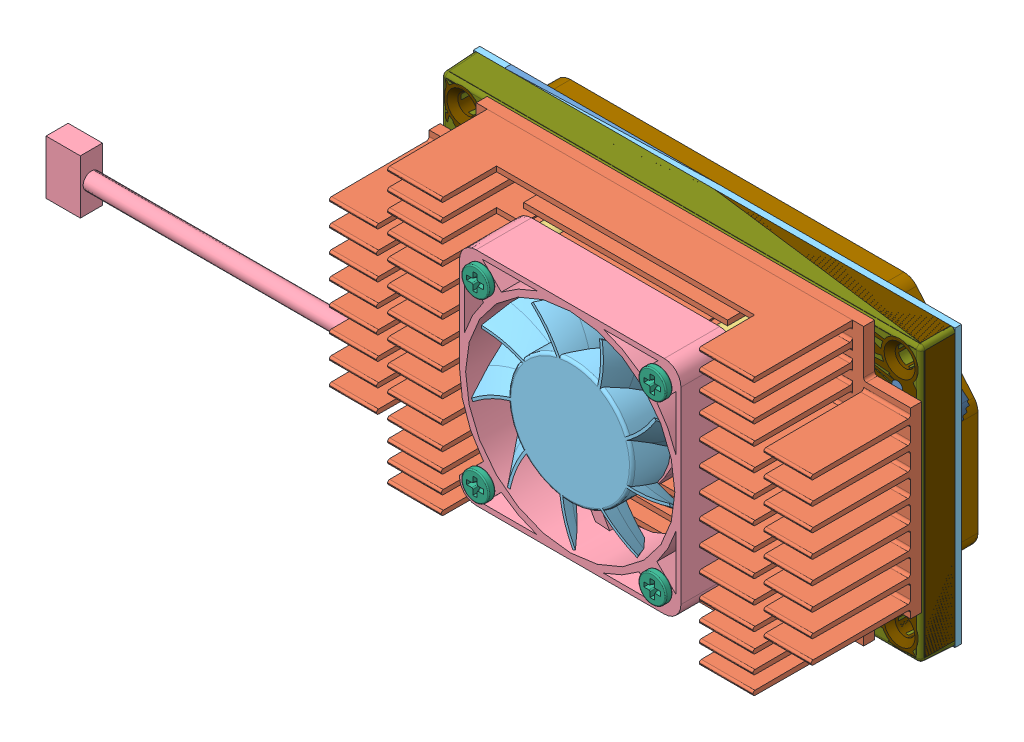
SolidWorks assembly JETSON-NEW_ASM, configuration Default. Lengths in mm. (continued)
Components (placement in the parent): (continued)
- 244-82180-1000-A01-07-31-15_ASM-1: 244-82180-1000-A01-07-31-15_ASM [Default] at origin size (87 50 8.3) (continued)
  - 039-0145-000_2-6: 039-0145-000_2 [Default] at (33.873 25.024 0) x (1 0 0) z (0 0 -1) size (1.4 0.7 0.62)
  - 039-0145-000_2-7: 039-0145-000_2 [Default] at (33.503 23.754 0) x (0 1 0) z (0 0 -1) size (1.4 0.7 0.62)
  - 039-0145-000_2-8: 039-0145-000_2 [Default] at (36.784 26.168 0) x (0 1 0) z (0 0 -1) size (1.4 0.7 0.62)
  - 039-0145-000_2-9: 039-0145-000_2 [Default] at (38.374 24.389 0) x (-1 0 0) z (0 0 -1) size (1.4 0.7 0.62)
  - 039-0188-000_3-5: 039-0188-000_3 [Default] at (36.3 38.2 0) x (-1 0 0) z (0 0 -1) size (1.4 0.7 0.67)
  - 039-0188-000_3-6: 039-0188-000_3 [Default] at (36.25 36.2 0) x (-1 0 0) z (0 0 -1) size (1.4 0.7 0.67)
  - 039-0188-000_3-7: 039-0188-000_3 [Default] at (36.9 32.05 0) x (-1 0 0) z (0 0 -1) size (1.4 0.7 0.67)
  - 039-0188-000_3-8: 039-0188-000_3 [Default] at (39.373 40.784 0) x (0 -1 0) z (0 0 -1) size (1.4 0.7 0.67)
  - 039-0145-000_2-10: 039-0145-000_2 [Default] at (39.753 24.004 0) x (0 1 0) z (0 0 -1) size (1.4 0.7 0.62)
  - 039-0145-000_2-11: 039-0145-000_2 [Default] at (39.495 25.352 0) x (1 0 0) z (0 0 -1) size (1.4 0.7 0.62)
  - 039-0188-000_3-9: 039-0188-000_3 [Default] at (38.003 41.604 0) x (0 1 0) z (0 0 -1) size (1.4 0.7 0.67)
  - 039-0145-000_2-12: 039-0145-000_2 [Default] at (41.353 24.824 0) x (0 1 0) z (0 0 -1) size (1.4 0.7 0.62)
  - 039-0145-000_2-13: 039-0145-000_2 [Default] at (43.188 24.838 0) x (0 1 0) z (0 0 -1) size (1.4 0.7 0.62)
  - 039-0145-000_2-14: 039-0145-000_2 [Default] at (42.268 24.828 0) x (0 1 0) z (0 0 -1) size (1.4 0.7 0.62)
  - 039-0145-000_2-15: 039-0145-000_2 [Default] at (42.863 23.214 0) x (1 0 0) z (0 0 -1) size (1.4 0.7 0.62)
  - 039-0197-000_3-1: 039-0197-000_3 [Default] at (48.75 34.85 0) x (1 0 0) z (0 0 -1) size (1.4 0.7 0.72)
  - 039-0197-000_3-2: 039-0197-000_3 [Default] at (47.5 35.75 0) x (1 0 0) z (0 0 -1) size (1.4 0.7 0.72)
  - 039-0188-000_3-10: 039-0188-000_3 [Default] at (45.093 41.024 0) x (1 0 0) z (0 0 -1) size (1.4 0.7 0.67)
  - 039-0197-000_3-3: 039-0197-000_3 [Default] at (45.9 35.75 0) x (-1 0 0) z (0 0 -1) size (1.4 0.7 0.72)
  - 039-0188-000_3-11: 039-0188-000_3 [Default] at (44.443 37.824 0) x (0 1 0) z (0 0 -1) size (1.4 0.7 0.67)
  - 039-0188-000_3-12: 039-0188-000_3 [Default] at (44.45 35.1 0) x (0 -1 0) z (0 0 -1) size (1.4 0.7 0.67)
  - 039-0188-000_3-13: 039-0188-000_3 [Default] at (11.15 20.65 0) x (0 1 0) z (0 0 -1) size (1.4 0.7 0.67)
  - 039-0145-000_2-16: 039-0145-000_2 [Default] at (11.607 27.979 1.164) x (-1 0 0) z (0 0 1) size (1.4 0.7 0.62)
  - 039-0145-000_2-17: 039-0145-000_2 [Default] at (16.618 28.397 1.164) size (1.4 0.7 0.62)
  - 039-0145-000_2-18: 039-0145-000_2 [Default] at (28.65 14.4 0) x (0 -1 0) z (0 0 -1) size (1.4 0.7 0.62)
  - 039-0145-000_2-19: 039-0145-000_2 [Default] at (6.05 21.2 0) x (-1 0 0) z (0 0 -1) size (1.4 0.7 0.62)
  - 039-0145-000_2-20: 039-0145-000_2 [Default] at (29.763 16.794 0) x (0 1 0) z (0 0 -1) size (1.4 0.7 0.62)
  - 039-0145-000_2-21: 039-0145-000_2 [Default] at (29.933 14.994 0) x (-1 0 0) z (0 0 -1) size (1.4 0.7 0.62)
  - 039-0145-000_2-22: 039-0145-000_2 [Default] at (28.85 20.15 0) x (1 0 0) z (0 0 -1) size (1.4 0.7 0.62)
  - 039-0145-000_2-23: 039-0145-000_2 [Default] at (31.063 15.984 0) x (-1 0 0) z (0 0 -1) size (1.4 0.7 0.62)
  - 039-0145-000_2-24: 039-0145-000_2 [Default] at (31.063 16.894 0) x (-1 0 0) z (0 0 -1) size (1.4 0.7 0.62)
  - 039-0145-000_2-25: 039-0145-000_2 [Default] at (31.703 12.644 0) x (0 -1 0) z (0 0 -1) size (1.4 0.7 0.62)
  - 039-0145-000_2-26: 039-0145-000_2 [Default] at (30.443 12.584 0) x (-1 0 0) z (0 0 -1) size (1.4 0.7 0.62)
  - 039-0145-000_2-27: 039-0145-000_2 [Default] at (30.443 13.484 0) x (-1 0 0) z (0 0 -1) size (1.4 0.7 0.62)
  - 039-0145-000_2-28: 039-0145-000_2 [Default] at (33 11.85 0) x (1 0 0) z (0 0 -1) size (1.4 0.7 0.62)
  - 039-0145-000_2-29: 039-0145-000_2 [Default] at (29.75 11.65 0) x (-1 0 0) z (0 0 -1) size (1.4 0.7 0.62)
  - 039-0145-000_2-30: 039-0145-000_2 [Default] at (29.413 21.065 0) x (1 0 0) z (0 0 -1) size (1.4 0.7 0.62)
  - 039-0145-000_2-31: 039-0145-000_2 [Default] at (34.423 13.174 0) x (0 -1 0) z (0 0 -1) size (1.4 0.7 0.62)
  - 039-0188-000_3-14: 039-0188-000_3 [Default] at (35.323 13.174 0) x (0 -1 0) z (0 0 -1) size (1.4 0.7 0.67)
  - 039-0145-000_2-32: 039-0145-000_2 [Default] at (34.963 11.574 0) x (0 -1 0) z (0 0 -1) size (1.4 0.7 0.62)
  - 039-0145-000_2-33: 039-0145-000_2 [Default] at (32.323 18.454 0) x (0 -1 0) z (0 0 -1) size (1.4 0.7 0.62)
  - 039-0145-000_2-34: 039-0145-000_2 [Default] at (33.523 13.124 0) x (0 -1 0) z (0 0 -1) size (1.4 0.7 0.62)
  - 039-0145-000_2-35: 039-0145-000_2 [Default] at (32.623 13.124 0) x (0 -1 0) z (0 0 -1) size (1.4 0.7 0.62)
  - 039-0145-000_2-36: 039-0145-000_2 [Default] at (30.888 22.484 0) x (-1 0 0) z (0 0 -1) size (1.4 0.7 0.62)
  - 039-0145-000_2-37: 039-0145-000_2 [Default] at (31.043 21.054 0) x (-1 0 0) z (0 0 -1) size (1.4 0.7 0.62)
  - 039-0145-000_2-38: 039-0145-000_2 [Default] at (31.063 19.634 0) x (-1 0 0) z (0 0 -1) size (1.4 0.7 0.62)
  - 039-0145-000_2-39: 039-0145-000_2 [Default] at (31.063 18.724 0) x (-1 0 0) z (0 0 -1) size (1.4 0.7 0.62)
  - 039-0145-000_2-40: 039-0145-000_2 [Default] at (31.063 17.794 0) x (-1 0 0) z (0 0 -1) size (1.4 0.7 0.62)
  - 039-0145-000_2-41: 039-0145-000_2 [Default] at (38.263 21.414 0) x (0 -1 0) z (0 0 -1) size (1.4 0.7 0.62)
  - 039-0145-000_2-42: 039-0145-000_2 [Default] at (37.353 21.374 0) x (0 -1 0) z (0 0 -1) size (1.4 0.7 0.62)
  - 039-0145-000_2-43: 039-0145-000_2 [Default] at (38.803 19.694 0) x (0 -1 0) z (0 0 -1) size (1.4 0.7 0.62)
  - 039-0145-000_2-44: 039-0145-000_2 [Default] at (37.853 19.694 0) x (0 -1 0) z (0 0 -1) size (1.4 0.7 0.62)
  - 039-0145-000_2-45: 039-0145-000_2 [Default] at (38.758 15.717 0) x (0 -1 0) z (0 0 -1) size (1.4 0.7 0.62)
  - 039-0145-000_2-46: 039-0145-000_2 [Default] at (37.846 15.717 0) x (0 -1 0) z (0 0 -1) size (1.4 0.7 0.62)
  - 039-0145-000_2-47: 039-0145-000_2 [Default] at (33.659 19.074 0) x (1 0 0) z (0 0 -1) size (1.4 0.7 0.62)
  - 039-0145-000_2-48: 039-0145-000_2 [Default] at (38.723 13.214 0) x (0 -1 0) z (0 0 -1) size (1.4 0.7 0.62)
  - 039-0145-000_2-49: 039-0145-000_2 [Default] at (38.003 11.924 0) x (1 0 0) z (0 0 -1) size (1.4 0.7 0.62)
  - 039-0145-000_2-50: 039-0145-000_2 [Default] at (36.073 19.694 0) x (0 -1 0) z (0 0 -1) size (1.4 0.7 0.62)
  - 039-0145-000_2-51: 039-0145-000_2 [Default] at (36.42 18.444 0) x (-1 0 0) z (0 0 -1) size (1.4 0.7 0.62)
  - 039-0145-000_2-52: 039-0145-000_2 [Default] at (36.42 16.644 0) x (-1 0 0) z (0 0 -1) size (1.4 0.7 0.62)
  - 039-0145-000_2-53: 039-0145-000_2 [Default] at (36.42 17.544 0) x (-1 0 0) z (0 0 -1) size (1.4 0.7 0.62)
  - 039-0145-000_2-54: 039-0145-000_2 [Default] at (37.123 13.174 0) x (0 -1 0) z (0 0 -1) size (1.4 0.7 0.62)
  - 039-0145-000_2-55: 039-0145-000_2 [Default] at (36.343 11.924 0) x (1 0 0) z (0 0 -1) size (1.4 0.7 0.62)
  - 039-0145-000_2-56: 039-0145-000_2 [Default] at (33.713 21.724 0) x (1 0 0) z (0 0 -1) size (1.4 0.7 0.62)
  - 039-0145-000_2-57: 039-0145-000_2 [Default] at (35.005 19.699 0) x (0 1 0) z (0 0 -1) size (1.4 0.7 0.62)
  - 039-0145-000_2-58: 039-0145-000_2 [Default] at (33.743 19.974 0) x (1 0 0) z (0 0 -1) size (1.4 0.7 0.62)
  - 039-0145-000_2-59: 039-0145-000_2 [Default] at (33.663 18.174 0) x (1 0 0) z (0 0 -1) size (1.4 0.7 0.62)
  - 039-0145-000_2-60: 039-0145-000_2 [Default] at (33.663 17.274 0) x (1 0 0) z (0 0 -1) size (1.4 0.7 0.62)
  - 039-0145-000_2-61: 039-0145-000_2 [Default] at (41.223 12.474 0) x (0 -1 0) z (0 0 -1) size (1.4 0.7 0.62)
  - 039-0145-000_2-62: 039-0145-000_2 [Default] at (42.133 12.464 0) x (0 -1 0) z (0 0 -1) size (1.4 0.7 0.62)
  - 039-0145-000_2-63: 039-0145-000_2 [Default] at (41.243 11.194 0) x (1 0 0) z (0 0 -1) size (1.4 0.7 0.62)
  - 039-0145-000_2-64: 039-0145-000_2 [Default] at (39.173 21.394 0) x (0 -1 0) z (0 0 -1) size (1.4 0.7 0.62)
  - 039-0145-000_2-65: 039-0145-000_2 [Default] at (40.513 19.724 0) x (0 -1 0) z (0 0 -1) size (1.4 0.7 0.62)
  - 039-0145-000_2-66: 039-0145-000_2 [Default] at (39.859 15.764 0) x (0 1 0) z (0 0 -1) size (1.4 0.7 0.62)
  - 039-0145-000_2-67: 039-0145-000_2 [Default] at (39.623 13.134 0) x (0 -1 0) z (0 0 -1) size (1.4 0.7 0.62)
  - 039-0145-000_2-68: 039-0145-000_2 [Default] at (39.973 11.514 0) x (0 -1 0) z (0 0 -1) size (1.4 0.7 0.62)
  - 039-0145-000_2-69: 039-0145-000_2 [Default] at (42.613 22.304 0) x (1 0 0) z (0 0 -1) size (1.4 0.7 0.62)
  - 039-0145-000_2-70: 039-0145-000_2 [Default] at (42.743 19.696 0) x (0 -1 0) z (0 0 -1) size (1.4 0.7 0.62)
  - 039-0145-000_2-71: 039-0145-000_2 [Default] at (42.143 17.394 0) x (1 0 0) z (0 0 -1) size (1.4 0.7 0.62)
  - 039-0145-000_2-72: 039-0145-000_2 [Default] at (42.163 16.484 0) x (1 0 0) z (0 0 -1) size (1.4 0.7 0.62)
  - 039-0145-000_2-73: 039-0145-000_2 [Default] at (42.183 15.564 0) x (1 0 0) z (0 0 -1) size (1.4 0.7 0.62)
  - 039-0145-000_2-74: 039-0145-000_2 [Default] at (42.163 14.634 0) x (1 0 0) z (0 0 -1) size (1.4 0.7 0.62)
  - 039-0145-000_2-75: 039-0145-000_2 [Default] at (43.033 13.374 0) x (0 1 0) z (0 0 -1) size (1.4 0.7 0.62)
  - 039-0145-000_2-76: 039-0145-000_2 [Default] at (40.433 21.064 0) x (-1 0 0) z (0 0 -1) size (1.4 0.7 0.62)
  - 039-0188-000_3-15: 039-0188-000_3 [Default] at (43.796 15.444 0) x (1 0 0) z (0 0 -1) size (1.4 0.7 0.67)
  - 039-0145-000_2-77: 039-0145-000_2 [Default] at (57 41.1 1.164) x (-1 0 0) z (0 0 1) size (1.4 0.7 0.62)
  - 039-0145-000_2-78: 039-0145-000_2 [Default] at (69.75 34.15 0) x (0 -1 0) z (0 0 -1) size (1.4 0.7 0.62)
  - 039-0188-000_3-16: 039-0188-000_3 [Default] at (72.05 30.95 0) x (-1 0 0) z (0 0 -1) size (1.4 0.7 0.67)
  - 039-0188-000_3-17: 039-0188-000_3 [Default] at (74.4 31.9 0) x (1 0 0) z (0 0 -1) size (1.4 0.7 0.67)
  - 039-0145-000_2-79: 039-0145-000_2 [Default] at (72.753 31.884 0) x (1 0 0) z (0 0 -1) size (1.4 0.7 0.62)
  - 039-0145-000_2-80: 039-0145-000_2 [Default] at (19.986 32.449 0) x (1 0 0) z (0 0 -1) size (1.4 0.7 0.62)
  - 039-0145-000_2-81: 039-0145-000_2 [Default] at (35.043 22.074 0) x (0 -1 0) z (0 0 -1) size (1.4 0.7 0.62)
  - 039-0145-000_2-82: 039-0145-000_2 [Default] at (29.622 22.319 0) x (0 1 0) z (0 0 -1) size (1.4 0.7 0.62)
  - 091-0022-000_1-1: 091-0022-000_1 [Default] at (69.45 12.65 0) x (1 0 0) z (0 0 -1) size (2 2.51 1.1)
  - 091-0022-000_1-2: 091-0022-000_1 [Default] at (59.9 10.85 1.164) x (0 1 0) z (0 0 1) size (2 2.51 1.1)
  - 300-0405-000_1-1: 300-0405-000_1 [Default] at (71.98 12.636 0) x (-1 0 0) z (0 0 -1) size (2 2.51 0.9)
  - 130-0580-000_4-1: 130-0580-000_4 [Default] at (59.063 24.389 1.164) x (-1 0 0) z (0 0 1) size (4.96 4.06 2)
  - 130-0580-000_4-2: 130-0580-000_4 [Default] at (59.063 15.039 1.164) x (-1 0 0) z (0 0 1) size (4.96 4.06 2)
  - 032-0470-000_2-1: 032-0470-000_2 [Default] at (69.75 32.2 0) x (0 -1 0) z (0 0 -1) size (2 0.84 0.97)
  - 032-0470-000_2-2: 032-0470-000_2 [Default] at (68.7 35.2 0) x (0 1 0) z (0 0 -1) size (2 0.84 0.97)
  - 032-0470-000_2-3: 032-0470-000_2 [Default] at (76.75 34.8 0) x (0 1 0) z (0 0 -1) size (2 0.84 0.97)
  - 032-0470-000_2-4: 032-0470-000_2 [Default] at (76.75 32.55 0) x (0 -1 0) z (0 0 -1) size (2 0.84 0.97)
  - 032-0421-000_2-1: 032-0421-000_2 [Default] at (67.6 18.85 1.164) x (-1 0 0) z (0 0 1) size (2 0.84 0.93)
  - 032-0421-000_2-2: 032-0421-000_2 [Default] at (72.4 14.7 1.164) size (2 0.84 0.93)
  - 032-0421-000_2-3: 032-0421-000_2 [Default] at (72.4 15.8 1.164) size (2 0.84 0.93)
  - 032-0421-000_2-4: 032-0421-000_2 [Default] at (72.4 16.9 1.164) size (2 0.84 0.93)
  - 032-0421-000_2-5: 032-0421-000_2 [Default] at (69.256 18.703 1.164) x (0 1 0) z (0 0 1) size (2 0.84 0.93)
  - 032-0421-000_2-6: 032-0421-000_2 [Default] at (71.8 26.54 1.164) x (0 1 0) z (0 0 1) size (2 0.84 0.93)
  - 032-0421-000_2-7: 032-0421-000_2 [Default] at (72.57 24.76 1.164) size (2 0.84 0.93)
  - 032-0421-000_2-8: 032-0421-000_2 [Default] at (72.593 21.459 1.164) size (2 0.84 0.93)
  - 032-0421-000_2-9: 032-0421-000_2 [Default] at (72.593 22.559 1.164) size (2 0.84 0.93)
  - 032-0421-000_2-10: 032-0421-000_2 [Default] at (72.593 23.659 1.164) size (2 0.84 0.93)
  - 032-0421-000_2-11: 032-0421-000_2 [Default] at (72.65 19.8 1.164) x (0 1 0) z (0 0 1) size (2 0.84 0.93)
  - 032-0421-000_2-12: 032-0421-000_2 [Default] at (70.61 25.68 1.164) x (0 1 0) z (0 0 1) size (2 0.84 0.93)
  - 032-0421-000_2-13: 032-0421-000_2 [Default] at (69.5 25.68 1.164) x (0 1 0) z (0 0 1) size (2 0.84 0.93)
  - 032-0421-000_2-14: 032-0421-000_2 [Default] at (71.553 19.804 1.164) x (0 1 0) z (0 0 1) size (2 0.84 0.93)
  - 032-0421-000_2-15: 032-0421-000_2 [Default] at (68.39 25.68 1.164) x (0 1 0) z (0 0 1) size (2 0.84 0.93)
  - 032-0421-000_2-16: 032-0421-000_2 [Default] at (70.35 19.8 1.164) x (0 1 0) z (0 0 1) size (2 0.84 0.93)
  - 036-0034-000_1-1: 036-0034-000_1 [Default] at (75.23 38.16 1.164) x (-1 0 0) z (0 0 1) size (2 0.84 1.02)
  - 036-0034-000_1-2: 036-0034-000_1 [Default] at (2.62 13.59 1.164) x (-1 0 0) z (0 0 1) size (2 0.84 1.02)
  - 039-0168-000_1-1: 039-0168-000_1 [Default] at (39.23 17.12 0) x (1 0 0) z (0 0 -1) size (2 0.84 0.92)
  - 039-0168-000_1-2: 039-0168-000_1 [Default] at (43.593 17.044 0) x (0 -1 0) z (0 0 -1) size (2 0.84 0.92)
  - 039-0168-000_1-3: 039-0168-000_1 [Default] at (45.6 19.3 0) x (0 1 0) z (0 0 -1) size (2 0.84 0.92)
  - 039-0168-000_1-4: 039-0168-000_1 [Default] at (46.75 19.3 0) x (0 1 0) z (0 0 -1) size (2 0.84 0.92)
  - 039-0168-000_1-5: 039-0168-000_1 [Default] at (44.693 17.044 0) x (0 -1 0) z (0 0 -1) size (2 0.84 0.92)
  - 039-0125-000_1-1: 039-0125-000_1 [Default] at (57.653 33.054 1.164) size (2 0.84 0.97)
  - 039-0125-000_1-2: 039-0125-000_1 [Default] at (58.453 14.204 0) x (0 -1 0) z (0 0 -1) size (2 0.84 0.97)
  - 032-0056-000_2-1: 032-0056-000_2 [Default] at (55.353 40.004 1.164) size (2 0.84 1.02)
  - 039-0125-000_1-3: 039-0125-000_1 [Default] at (55.67 36.86 1.164) x (0 -1 0) z (0 0 1) size (2 0.84 0.97)
  - 039-0125-000_1-4: 039-0125-000_1 [Default] at (55.67 34.6 1.164) x (0 1 0) z (0 0 1) size (2 0.84 0.97)
  - 032-0056-000_2-2: 032-0056-000_2 [Default] at (54.489 31.838 1.164) size (2 0.84 1.02)
  - 032-0056-000_2-3: 032-0056-000_2 [Default] at (55.145 29.717 1.164) x (0 1 0) z (0 0 1) size (2 0.84 1.02)
  - 039-0125-000_1-5: 039-0125-000_1 [Default] at (59.953 33.054 1.164) x (-1 0 0) z (0 0 1) size (2 0.84 0.97)
  - 032-0056-000_2-4: 032-0056-000_2 [Default] at (59.62 31.466 0) x (1 0 0) z (0 0 -1) size (2 0.84 1.02)
  - 039-0125-000_1-6: 039-0125-000_1 [Default] at (61.796 34.84 1.164) x (0 1 0) z (0 0 1) size (2 0.84 0.97)
  - 215-0151-000_1-1: 215-0151-000_1 [Default] at (61.52 33.156 0) x (1 0 0) z (0 0 -1) size (2 0.84 0.6)
  - 032-0056-000_2-5: 032-0056-000_2 [Default] at (61.873 31.574 1.164) x (-1 0 0) z (0 0 1) size (2 0.84 1.02)
  - 032-0056-000_2-6: 032-0056-000_2 [Default] at (62.63 29.916 1.164) x (0 -1 0) z (0 0 1) size (2 0.84 1.02)
  - 039-0125-000_1-7: 039-0125-000_1 [Default] at (65.253 22.254 0) x (-1 0 0) z (0 0 -1) size (2 0.84 0.97)
  - 039-0168-000_1-6: 039-0168-000_1 [Default] at (44.7 13.8 0) x (0 1 0) z (0 0 -1) size (2 0.84 0.92)
  - 039-0037-000_1-1: 039-0037-000_1 [Default] at (68.83 5.23 1.164) x (0 -1 0) z (0 0 1) size (2 0.84 1.02)
  - 039-0037-000_1-2: 039-0037-000_1 [Default] at (77.9 14.1 1.164) x (0 1 0) z (0 0 1) size (2 0.84 1.02)
  - 039-0037-000_1-3: 039-0037-000_1 [Default] at (75.8 4.05 1.164) size (2 0.84 1.02)
  - 195-1225-000_1-1: 195-1225-000_1 [Default] at (62.4 42.78 0) x (0 1 0) z (0 0 -1) size (2 0.84 0.62)
  - 195-1260-000_1-1: 195-1260-000_1 [Default] at (10.9 32.65 0) x (1 0 0) z (0 0 -1) size (2 0.84 0.62)
  - 036-0043-000_1-1: 036-0043-000_1 [Default] at (5.524 36.6 0) x (0 1 0) z (0 0 -1) size (2 0.84 1.02)
  - 100-0104-000_1-1: 100-0104-000_1 [Default] at (28.2 15.55 0) x (1 0 0) z (0 0 -1) size (1.75 0.53 0.5)
  - 100-0063-000_1-1: 100-0063-000_1 [Default] at (21.1 20.85 1.164) x (-1 0 0) z (0 0 1) size (1.75 0.53 0.55)
  - 100-0063-000_1-2: 100-0063-000_1 [Default] at (45.21 8.116 1.164) size (1.75 0.53 0.55)
  - 100-0063-000_1-3: 100-0063-000_1 [Default] at (21.8 29.4 1.164) x (0 1 0) z (0 0 1) size (1.75 0.53 0.55)
  - 100-0063-000_1-4: 100-0063-000_1 [Default] at (27.15 25.1 1.164) x (-1 0 0) z (0 0 1) size (1.75 0.53 0.55)
  - 100-0063-000_1-5: 100-0063-000_1 [Default] at (27.713 20.824 1.164) x (0 1 0) z (0 0 1) size (1.75 0.53 0.55)
  - 100-0063-000_1-6: 100-0063-000_1 [Default] at (32.232 9.282 1.164) size (1.75 0.53 0.55)
  - 100-0104-000_1-2: 100-0104-000_1 [Default] at (28.8 19.25 0) x (1 0 0) z (0 0 -1) size (1.75 0.53 0.5)
  - 100-0104-000_1-3: 100-0104-000_1 [Default] at (33.6 11.05 0) x (1 0 0) z (0 0 -1) size (1.75 0.53 0.5)
  - 100-0063-000_1-7: 100-0063-000_1 [Default] at (33.943 9.709 1.164) x (0 -1 0) z (0 0 1) size (1.75 0.53 0.55)
  - 100-0189-000_2-1: 100-0189-000_2 [Default] at (43.113 20.934 0) x (1 0 0) z (0 0 -1) size (1.75 0.53 0.55)
  - 100-0063-000_1-8: 100-0063-000_1 [Default] at (46.76 10.216 1.164) size (1.75 0.53 0.55)
  - 100-0189-000_2-2: 100-0189-000_2 [Default] at (22.95 25.35 1.164) x (-1 0 0) z (0 0 1) size (1.75 0.53 0.55)
  - 100-0063-000_1-9: 100-0063-000_1 [Default] at (46.93 23.266 1.164) size (1.75 0.53 0.55)
  - 100-0165-000_1-1: 100-0165-000_1 [Default] at (73.7 12.5 0) x (0 -1 0) z (0 0 -1) size (1.75 0.53 0.6)
  - 039-0122-000_1-1: 039-0122-000_1 [Default] at (53.84 22.3 0) x (0 -1 0) z (0 0 -1) size (3.05 1.27 0.95)
  - 039-0122-000_1-2: 039-0122-000_1 [Default] at (55.93 22.35 0) x (0 -1 0) z (0 0 -1) size (3.05 1.27 0.95)
  - 032-0037-000_2-1: 032-0037-000_2 [Default] at (47.8 13.8 0) x (1 0 0) z (0 0 -1) size (3.05 1.27 0.95)
  - 032-0037-000_2-2: 032-0037-000_2 [Default] at (40.15 26.75 0) x (1 0 0) z (0 0 -1) size (3.05 1.27 0.95)
  - 039-0122-000_1-3: 039-0122-000_1 [Default] at (47.153 31.164 0) x (0 1 0) z (0 0 -1) size (3.05 1.27 0.95)
  - 039-0122-000_1-4: 039-0122-000_1 [Default] at (48.803 31.154 0) x (0 1 0) z (0 0 -1) size (3.05 1.27 0.95)
  - 039-0122-000_1-5: 039-0122-000_1 [Default] at (47.278 13.804 1.164) x (0 -1 0) z (0 0 1) size (3.05 1.27 0.95)
  - 032-0037-000_2-3: 032-0037-000_2 [Default] at (47.778 15.548 0) x (1 0 0) z (0 0 -1) size (3.05 1.27 0.95)
  - 032-0037-000_2-4: 032-0037-000_2 [Default] at (48.978 13.804 1.164) x (0 -1 0) z (0 0 1) size (3.05 1.27 0.95)
  - 039-0122-000_1-6: 039-0122-000_1 [Default] at (49.67 20.36 0) x (1 0 0) z (0 0 -1) size (3.05 1.27 0.95)
  - 032-0037-000_2-5: 032-0037-000_2 [Default] at (47.778 17.15 0) x (1 0 0) z (0 0 -1) size (3.05 1.27 0.95)
  - 032-0037-000_2-6: 032-0037-000_2 [Default] at (50.678 13.804 1.164) x (0 -1 0) z (0 0 1) size (3.05 1.27 0.95)
  - 039-0122-000_1-7: 039-0122-000_1 [Default] at (59.544 23.53 0) x (1 0 0) z (0 0 -1) size (3.05 1.27 0.95)
  - 039-0122-000_1-8: 039-0122-000_1 [Default] at (57.95 28.15 1.164) size (3.05 1.27 0.95)
  - 039-0122-000_1-9: 039-0122-000_1 [Default] at (59.515 25.132 0) x (1 0 0) z (0 0 -1) size (3.05 1.27 0.95)
  - 039-0122-000_1-10: 039-0122-000_1 [Default] at (59.483 28.504 0) x (1 0 0) z (0 0 -1) size (3.05 1.27 0.95)
  - 039-0122-000_1-11: 039-0122-000_1 [Default] at (59.483 26.754 0) x (1 0 0) z (0 0 -1) size (3.05 1.27 0.95)
  - 039-0122-000_1-12: 039-0122-000_1 [Default] at (59.483 30.134 0) x (1 0 0) z (0 0 -1) size (3.05 1.27 0.95)
  - 215-0165-000_1-1: 215-0165-000_1 [Default] at (73.833 26.174 1.164) size (3.05 1.27 0.6)
  - 215-0165-000_1-2: 215-0165-000_1 [Default] at (74.004 19.147 1.164) x (0 1 0) z (0 0 1) size (3.05 1.27 0.6)
  - 032-0213-000_1-1: 032-0213-000_1 [Default] at (12.3 38.75 0) x (1 0 0) z (0 0 -1) size (3.05 1.27 1.45)
  - 100-0077-000_1-1: 100-0077-000_1 [Default] at (16.393 37.444 1.164) x (-1 0 0) z (0 0 1) size (2.22 0.81 0.95)
  - 085-0232-000_1-1: 085-0232-000_1 [Default] at (66.12 7.63 1.164) x (-1 0 0) z (0 0 1) size (3.81 2.5 0.75)
  - 161-0188-600_2-1: 161-0188-600_2 [Default] at (28.903 37.199 1.164) x (0 1 0) z (0 0 1) size (10.1 15.1 1)
  - 161-0188-600_2-2: 161-0188-600_2 [Default] at (44.603 37.199 1.164) x (0 1 0) z (0 0 1) size (10.1 15.1 1)
  - 300-0868-000_3-1: 300-0868-000_3 [Default] at (53.3 9.55 1.164) size (1 0.6 0.41)
  - 300-0868-000_3-2: 300-0868-000_3 [Default] at (15.5 12.85 0) x (-1 0 0) z (0 0 -1) size (1 0.6 0.41)
  - 300-0868-000_3-3: 300-0868-000_3 [Default] at (71 25.95 0) x (1 0 0) z (0 0 -1) size (1 0.6 0.41)
  - 300-0868-000_3-4: 300-0868-000_3 [Default] at (63.182 37.401 0) x (0 1 0) z (0 0 -1) size (1 0.6 0.41)
  - 300-0870-000_1-1: 300-0870-000_1 [Default] at (31.482 11.077 0) x (-1 0 0) z (0 0 -1) size (1 0.6 0.41)
  - 131-0632-000_2-1: 131-0632-000_2 [Default] at (72.11 12.9 1.164) size (3.05 1.27 1.4)
  - 300-0494-000_1-1: 300-0494-000_1 [Default] at (71.55 15.75 0) x (1 0 0) z (0 0 -1) size (2.94 3.2 1.21)
  - 305-0002-000_1-1: 305-0002-000_1 [Default] at (7.2 38.8 0) x (1 0 0) z (0 0 -1) size (2.94 3.2 1.12)
  - 091-0004-000_1-1: 091-0004-000_1 [Default] at (10.4 42.15 0) x (-1 0 0) z (0 0 -1) size (2.94 3.2 1.27)
  - 300-0329-000_1-1: 300-0329-000_1 [Default] at (72.34 28.306 0) x (1 0 0) z (0 0 -1) size (2.94 3.2 1.26)
  - 300-0329-000_1-2: 300-0329-000_1 [Default] at (64.59 42.16 0) x (-1 0 0) z (0 0 -1) size (2.94 3.2 1.26)
  - 300-0329-000_1-3: 300-0329-000_1 [Default] at (56.09 12.826 0) x (-1 0 0) z (0 0 -1) size (2.94 3.2 1.26)
  - 300-0329-000_1-4: 300-0329-000_1 [Default] at (65.57 37.196 0) x (1 0 0) z (0 0 -1) size (2.94 3.2 1.26)
  - 300-0329-000_1-5: 300-0329-000_1 [Default] at (65.72 33.816 0) x (0 -1 0) z (0 0 -1) size (2.94 3.2 1.26)
  - 300-0329-000_1-6: 300-0329-000_1 [Default] at (62.55 12.6 0) x (0 1 0) z (0 0 -1) size (2.94 3.2 1.26)
  - 300-0329-000_1-7: 300-0329-000_1 [Default] at (10.54 35.996 0) x (1 0 0) z (0 0 -1) size (2.94 3.2 1.26)
  - 080-0550-000_2-1: 080-0550-000_2 [Default] at (-1.294 28.232 1.164) x (0 1 0) z (0 0 1) size (3.63 4.07 1.47)
  - 080-0550-000_2-2: 080-0550-000_2 [Default] at (-1.294 33.789 1.164) x (0 1 0) z (0 0 1) size (3.63 4.07 1.47)
  - SAMTEC-SEAF-50-05-S-08-02-A-K_ASM-1: SAMTEC-SEAF-50-05-S-08-02-A-K_ASM [Default] at (39.4993 3.4 -0.7366) x (0 -1 0) z (1 0 0) size (10.74 6.33 70.16)
    - SAMTEC-JETSON_ASM-1: SAMTEC-JETSON_ASM [Default] at origin size (10.74 6.33 70.16)
      - BOSS-BASE-1: BOSS-BASE [Default] at origin size (10.74 6.33 70.16)
- 244-82180-1000-A03-10-12-15_ASM-1: 244-82180-1000-A03-10-12-15_ASM [Default] at origin size (87 50 8.3)
  - 142-82180-1000-A03-10-12-15-1: 142-82180-1000-A03-10-12-15 [Default] at origin size (87 50 1.16)
  - 032-0628-000_1-1: 032-0628-000_1 [Default] at (13.96 6.5 1.164) x (0 1 0) z (0 0 1) size (3.82 1.6 1.8)
  - 032-0628-000_1-2: 032-0628-000_1 [Default] at (11.83 6.48 1.164) x (0 1 0) z (0 0 1) size (3.82 1.6 1.8)
  - 032-0628-000_1-3: 032-0628-000_1 [Default] at (55.94 22.44 0) x (0 -1 0) z (0 0 -1) size (3.82 1.6 1.8)
  - 032-0628-000_1-4: 032-0628-000_1 [Default] at (53.83 22.43 0) x (0 -1 0) z (0 0 -1) size (3.82 1.6 1.8)
  - 032-0637-000_1-1: 032-0637-000_1 [Default] at (72.8 32.06 1.164) size (3.82 1.6 1.8)
  - 032-0637-000_1-2: 032-0637-000_1 [Default] at (72.8 30 1.164) size (3.82 1.6 1.8)
  - 032-0471-000_2-1: 032-0471-000_2 [Default] at (49.67 19.576 0) x (1 0 0) z (0 0 -1) size (4.22 2.82 1.2)
  - 032-0471-000_2-2: 032-0471-000_2 [Default] at (36.91 17.143 0) x (-1 0 0) z (0 0 -1) size (4.22 2.82 1.2)
  - 032-0681-000_1-1: 032-0681-000_1 [Default] at (54.36 22.056 0) x (0 -1 0) z (0 0 -1) size (4.22 2.82 2)
  - 032-0681-000_1-2: 032-0681-000_1 [Default] at (47.78 16.326 0) x (1 0 0) z (0 0 -1) size (4.22 2.82 2)
  - 032-0681-000_1-3: 032-0681-000_1 [Default] at (47.778 13.049 0) x (1 0 0) z (0 0 -1) size (4.22 2.82 2)
  - 032-0627-000_1-1: 032-0627-000_1 [Default] at (1.38 11.27 1.164) x (-1 0 0) z (0 0 1) size (4.22 2.82 1.2)
  - 032-0627-000_1-2: 032-0627-000_1 [Default] at (72.09 40.46 1.164) size (4.22 2.82 1.2)
  - 032-0627-000_1-3: 032-0627-000_1 [Default] at (68.106 40.15 1.164) x (0 -1 0) z (0 0 1) size (4.22 2.82 1.2)
  - 032-0627-000_1-4: 032-0627-000_1 [Default] at (1.38 7.93 1.164) x (-1 0 0) z (0 0 1) size (4.22 2.82 1.2)
  - 041-0210-000_1-1: 041-0210-000_1 [Default] at (58.51 28.426 0) x (1 0 0) z (0 0 -1) size (8.63 4.4 1.22)
  - 041-0210-000_1-2: 041-0210-000_1 [Default] at (49.99 14.669 0) x (1 0 0) z (0 0 -1) size (8.63 4.4 1.22)
  - 041-0210-000_1-3: 041-0210-000_1 [Default] at (54.05 33.296 0) x (1 0 0) z (0 0 -1) size (8.63 4.4 1.22)
  - 041-0210-000_1-4: 041-0210-000_1 [Default] at (49.2 15.086 1.164) x (0 -1 0) z (0 0 1) size (8.63 4.4 1.22)
  - 090-0212-000_1-1: 090-0212-000_1 [Default] at (55.8 37.95 0) x (-1 0 0) z (0 0 -1) size (2.12 0.8 0.65)
  - 090-0283-000_3-1: 090-0283-000_3 [Default] at (62.7 14.85 0) x (0 1 0) z (0 0 -1) size (1.41 0.61 0.4)
  - 300-0688-000_1-1: 300-0688-000_1 [Default] at (56.25 13.65 0) x (-1 0 0) z (0 0 -1) size (1.21 1.41 0.55)
  - 300-0688-000_1-2: 300-0688-000_1 [Default] at (72.9 24.95 0) x (-1 0 0) z (0 0 -1) size (1.21 1.41 0.55)
  - 300-0688-000_1-3: 300-0688-000_1 [Default] at (8.7 35.95 0) x (0 1 0) z (0 0 -1) size (1.21 1.41 0.55)
  - 300-0688-000_1-4: 300-0688-000_1 [Default] at (60.55 12.2 0) x (0 1 0) z (0 0 -1) size (1.21 1.41 0.55)
  - 300-0688-000_1-5: 300-0688-000_1 [Default] at (58.95 12.05 0) x (1 0 0) z (0 0 -1) size (1.21 1.41 0.55)
  - 300-0688-000_1-6: 300-0688-000_1 [Default] at (65.15 11.55 0) x (0 -1 0) z (0 0 -1) size (1.21 1.41 0.55)
  - 316-0254-000_2-1: 316-0254-000_2 [Default] at (68.553 22.011 0) x (1 0 0) z (0 0 -1) size (3.51 3.51 0.8)
  - 316-0254-000_2-2: 316-0254-000_2 [Default] at (58.553 17.504 0) x (0 1 0) z (0 0 -1) size (3.51 3.51 0.8)
  - RES_04_SMD_015X032_0750_GREY-1: RES_04_SMD_015X032_0750_GREY [Default] at (12.96 1.05 1.164) x (0 -1 0) z (0 0 1) size (2.76 3.51 0.75)
  - QFN048Q_P040_0060_T045X04__GREY-1: QFN048Q_P040_0060_T045X04__GREY [Default] at (74.15 8.8 1.164) x (0 1 0) z (0 0 1) size (6 6 1)
  - 320-1075-000_1-1: 320-1075-000_1 [Default] at (5.85 26.7 1.164) x (-1 0 0) z (0 0 1) size (4.5 0.8 0.86)
  - 320-1075-000_1-2: 320-1075-000_1 [Default] at (16.1 38.75 1.164) size (4.5 0.8 0.86)
  - 320-1075-000_1-3: 320-1075-000_1 [Default] at (20.1 32.7 1.164) x (0 1 0) z (0 0 1) size (4.5 0.8 0.86)
  - 320-1075-000_1-4: 320-1075-000_1 [Default] at (16.1 26.7 1.164) x (-1 0 0) z (0 0 1) size (4.5 0.8 0.86)
  - 320-1075-000_1-5: 320-1075-000_1 [Default] at (5.85 38.75 1.164) size (4.5 0.8 0.86)
  - 320-1075-000_1-6: 320-1075-000_1 [Default] at (1.45 33.95 1.164) x (0 1 0) z (0 0 1) size (4.5 0.8 0.86)
  - 101-0104-000_2-1: 101-0104-000_2 [Default] at (3.212 36.749 1.164) x (0 1 0) z (0 0 1) size (2.02 1.5 1.01)
  - 101-0104-000_2-2: 101-0104-000_2 [Default] at (3.212 31.163 1.164) x (0 1 0) z (0 0 1) size (2.02 1.5 1.01)
  - T210-INT-DSC-A1_1_GREY-1: T210-INT-DSC-A1_1_GREY [Default] at (36.553 18.804 1.164) size (16.2 16.2 1)
  - 115-1605-000_1-1: 115-1605-000_1 [Default] at (67.968 40.894 0) x (0 -1 0) z (0 0 -1) size (2.51 2.01 0.41)
  - 080-1277-000_4_GREY-1: 080-1277-000_4_GREY [Default] at (39.5 3.4 0) x (1 0 0) z (0 0 -1) size (70.16 10.74 6.33)
  - 115-1265-000_1_GREY-1: 115-1265-000_1_GREY [Default] at (25.202 12.934 0) x (-1 0 0) z (0 0 -1) size (0.96 0.96 0.33)
  - 115-1265-000_1_GREY-2: 115-1265-000_1_GREY [Default] at (24.482 16.764 0) x (-1 0 0) z (0 0 -1) size (0.96 0.96 0.33)
  - 316-0420-000_3-1: 316-0420-000_3 [Default] at (6.32 10.69 1.164) size (3.5 3.5 1)
  - 316-0420-000_3-2: 316-0420-000_3 [Default] at (73.91 35.696 1.164) x (0 -1 0) z (0 0 1) size (3.5 3.5 1)
  - 130-0693-000_1-1: 130-0693-000_1 [Default] at (67.584 34.59 1.164) x (0 -1 0) z (0 0 1) size (6.2 4.9 1.8)
  - 130-0692-000_1-1: 130-0692-000_1 [Default] at (7.39 4.464 1.164) size (6.2 4.9 1.8)
  - 115-1066-000_2-1: 115-1066-000_2 [Default] at (72.703 34.834 0) x (1 0 0) z (0 0 -1) size (4.59 4.59 1)
  - 115-1272-000_1_GREY-1: 115-1272-000_1_GREY [Default] at (19.03 31.279 0) x (0 1 0) z (0 0 -1) size (0.76 0.76 0.39)
  - 115-1272-000_1_GREY-2: 115-1272-000_1_GREY [Default] at (14.95 40.6 0) x (0 1 0) z (0 0 -1) size (0.76 0.76 0.39)
  - 115-1156-000_1-1: 115-1156-000_1 [Default] at (49.173 28.444 0) x (0 -1 0) z (0 0 -1) size (2 2.5 0.8)
  - 115-1659-000_1-1: 115-1659-000_1 [Default] at (15.353 33.154 1.164) x (0 -1 0) z (0 0 1) size (4.87 7.71 0.31)
  - 115-1264-000_1-1: 115-1264-000_1 [Default] at (5.393 34.434 1.164) x (-1 0 0) z (0 0 1) size (1.2 1.2 0.51)
  - 115-1264-000_1-2: 115-1264-000_1 [Default] at (8.309 31.804 1.164) x (-1 0 0) z (0 0 1) size (1.2 1.2 0.51)
  - 115-1264-000_1-3: 115-1264-000_1 [Default] at (7.013 29.684 1.164) x (-1 0 0) z (0 0 1) size (1.2 1.2 0.51)
  - 115-1263-000_1-1: 115-1263-000_1 [Default] at (8.897 36.999 1.164) size (2.01 1.5 0.5)
  - 315-0931-000_1_GREY-1: 315-0931-000_1_GREY [Default] at (58.803 35.664 1.164) size (4.08 3.78 0.45)
  - 115-0880-000_1-1: 115-0880-000_1 [Default] at (48.278 39.304 0) x (1 0 0) z (0 0 -1) size (3 5.85 1.1)
  - 170-0212-000_2_GREY-1: 170-0212-000_2_GREY [Default] at (10.6 18.8 1.164) x (0 -1 0) z (0 0 1) size (11.5 13 0.48)
  - 174-0165-000_1-1: 174-0165-000_1 [Default] at (18.058 40.074 0) x (1 0 0) z (0 0 -1) size (2 3.52 0.55)
  - 032-0421-000_3-1: 032-0421-000_3 [Default] at (66.8 18.85 1.164) x (-1 0 0) z (0 0 1) size (2.2 1 1)
  - 032-0421-000_3-2: 032-0421-000_3 [Default] at (72.4 14.5 1.164) size (2.2 1 1)
  - 032-0421-000_3-3: 032-0421-000_3 [Default] at (72.4 15.75 1.164) size (2.2 1 1)
  - 032-0421-000_3-4: 032-0421-000_3 [Default] at (72.4 17 1.164) size (2.2 1 1)
  - 032-0421-000_3-5: 032-0421-000_3 [Default] at (68.656 18.703 1.164) x (0 1 0) z (0 0 1) size (2.2 1 1)
  - 032-0421-000_3-6: 032-0421-000_3 [Default] at (72 26.94 1.164) x (0 1 0) z (0 0 1) size (2.2 1 1)
  - 032-0421-000_3-7: 032-0421-000_3 [Default] at (72.57 24.96 1.164) size (2.2 1 1)
  - 032-0421-000_3-8: 032-0421-000_3 [Default] at (72.593 21.159 1.164) size (2.2 1 1)
  - 032-0421-000_3-9: 032-0421-000_3 [Default] at (72.593 22.409 1.164) size (2.2 1 1)
  - 032-0421-000_3-10: 032-0421-000_3 [Default] at (72.593 23.659 1.164) size (2.2 1 1)
  - 032-0421-000_3-11: 032-0421-000_3 [Default] at (72.55 19.3 1.164) x (0 1 0) z (0 0 1) size (2.2 1 1)
  - 032-0421-000_3-12: 032-0421-000_3 [Default] at (70.61 25.78 1.164) x (0 1 0) z (0 0 1) size (2.2 1 1)
  - 032-0421-000_3-13: 032-0421-000_3 [Default] at (69.35 25.78 1.164) x (0 1 0) z (0 0 1) size (2.2 1 1)
  - 032-0421-000_3-14: 032-0421-000_3 [Default] at (71.253 19.304 1.164) x (0 1 0) z (0 0 1) size (2.2 1 1)
  - 032-0421-000_3-15: 032-0421-000_3 [Default] at (68.04 25.78 1.164) x (0 1 0) z (0 0 1) size (2.2 1 1)
  - 032-0421-000_3-16: 032-0421-000_3 [Default] at (69.95 19.3 1.164) x (0 1 0) z (0 0 1) size (2.2 1 1)
  - 215-0249-000_1-1: 215-0249-000_1 [Default] at (59.32 33.436 0) x (0 1 0) z (0 0 -1) size (2.2 1 0.7)
  - 085-0174-000_1-1: 085-0174-000_1 [Default] at (61.96 37.206 1.164) x (0 1 0) z (0 0 1) size (2.2 1.4 0.6)
  - 195-1636-000_1-1: 195-1636-000_1 [Default] at (62.55 39.25 0) x (0 1 0) z (0 0 -1) size (0.69 0.32 0.31)
  - 130-0360-000_1-1: 130-0360-000_1 [Default] at (3.503 32.979 1.164) x (-1 0 0) z (0 0 1) size (0.69 0.32 0.34)
  - 130-0360-000_1-2: 130-0360-000_1 [Default] at (4.55 36.748 1.164) x (0 -1 0) z (0 0 1) size (0.69 0.32 0.34)
  - 035-0156-000_1-1: 035-0156-000_1 [Default] at (57.75 12.3 0) x (0 -1 0) z (0 0 -1) size (0.69 0.32 0.34)
  - 130-0333-000_1-1: 130-0333-000_1 [Default] at (-1.8 31.15 1.164) x (-1 0 0) z (0 0 1) size (0.69 0.32 0.34)
  - 130-0333-000_1-2: 130-0333-000_1 [Default] at (-1.75 36.75 1.164) x (-1 0 0) z (0 0 1) size (0.69 0.32 0.34)
  - 130-0341-000_1-1: 130-0341-000_1 [Default] at (9.894 30.222 1.164) x (-1 0 0) z (0 0 1) size (0.69 0.32 0.34)
  - 032-0640-000_1-1: 032-0640-000_1 [Default] at (10.709 29.981 1.164) x (0 -1 0) z (0 0 1) size (0.69 0.32 0.34)
  - 195-2117-000_1-1: 195-2117-000_1 [Default] at (67.3 11.45 0) x (-1 0 0) z (0 0 -1) size (0.69 0.32 0.31)
  - 195-1636-000_1-2: 195-1636-000_1 [Default] at (68.5 29.95 0) x (-1 0 0) z (0 0 -1) size (0.69 0.32 0.31)
  - 195-1636-000_1-3: 195-1636-000_1 [Default] at (10.2 12.1 0) x (0 -1 0) z (0 0 -1) size (0.69 0.32 0.31)
  - 039-0120-000_1-1: 039-0120-000_1 [Default] at (71.15 26.95 0) x (0 1 0) z (0 0 -1) size (0.69 0.32 0.34)
  - 195-2006-000_1-1: 195-2006-000_1 [Default] at (19.3 24.5 0) x (0 1 0) z (0 0 -1) size (0.69 0.32 0.31)
  - 195-2006-000_1-2: 195-2006-000_1 [Default] at (20.35 21.9 0) x (1 0 0) z (0 0 -1) size (0.69 0.32 0.31)
  - 039-0165-000_1-1: 039-0165-000_1 [Default] at (70.54 37.626 0) x (0 1 0) z (0 0 -1) size (0.69 0.32 0.34)
  - 039-0165-000_1-2: 039-0165-000_1 [Default] at (66.428 40.056 0) x (0 -1 0) z (0 0 -1) size (0.69 0.32 0.34)
  - 195-1636-000_1-4: 195-1636-000_1 [Default] at (69.1 39.206 0) x (0 -1 0) z (0 0 -1) size (0.69 0.32 0.31)
  - 039-0161-000_1-1: 039-0161-000_1 [Default] at (68.56 39.206 0) x (0 -1 0) z (0 0 -1) size (0.69 0.32 0.34)
  - 035-0243-000_2-1: 035-0243-000_2 [Default] at (19.65 20.85 1.164) x (-1 0 0) z (0 0 1) size (0.69 0.32 0.34)
  - 130-0344-000_1-1: 130-0344-000_1 [Default] at (9.138 34.734 1.164) x (-1 0 0) z (0 0 1) size (0.69 0.32 0.34)
  - 195-1636-000_1-5: 195-1636-000_1 [Default] at (75.45 36.836 0) x (0 -1 0) z (0 0 -1) size (0.69 0.32 0.31)
  - 195-2034-000_1-1: 195-2034-000_1 [Default] at (30.5 10.1 1.164) x (0 -1 0) z (0 0 1) size (0.69 0.32 0.31)
  - 195-2034-000_1-2: 195-2034-000_1 [Default] at (47.3 23.95 1.164) size (0.69 0.32 0.31)
  - 195-1636-000_1-6: 195-1636-000_1 [Default] at (75.453 35.934 0) x (0 1 0) z (0 0 -1) size (0.69 0.32 0.31)
  - 195-1636-000_1-7: 195-1636-000_1 [Default] at (75.453 35.034 0) x (0 -1 0) z (0 0 -1) size (0.69 0.32 0.31)
  - 215-0247-000_1-1: 215-0247-000_1 [Default] at (77.75 33.95 0) x (1 0 0) z (0 0 -1) size (0.69 0.32 0.33)
  - 215-0247-000_1-2: 215-0247-000_1 [Default] at (74.5 30.85 0) x (1 0 0) z (0 0 -1) size (0.69 0.32 0.33)
  - 215-0247-000_1-3: 215-0247-000_1 [Default] at (68.7 33.75 0) x (1 0 0) z (0 0 -1) size (0.69 0.32 0.33)
  - 195-2118-000_1-1: 195-2118-000_1 [Default] at (58.9 8 1.164) x (0 -1 0) z (0 0 1) size (0.69 0.32 0.31)
  - 195-2118-000_1-2: 195-2118-000_1 [Default] at (57.55 8.25 1.164) x (-1 0 0) z (0 0 1) size (0.69 0.32 0.31)
  - 195-2118-000_1-3: 195-2118-000_1 [Default] at (58.3 8 1.164) x (0 -1 0) z (0 0 1) size (0.69 0.32 0.31)
  - 195-2005-000_1-1: 195-2005-000_1 [Default] at (16.46 40.946 0) x (-1 0 0) z (0 0 -1) size (0.69 0.32 0.31)
  - 195-2005-000_1-2: 195-2005-000_1 [Default] at (16.46 41.476 0) x (1 0 0) z (0 0 -1) size (0.69 0.32 0.31)
  - 195-2005-000_1-3: 195-2005-000_1 [Default] at (17.26 42.436 0) x (0 1 0) z (0 0 -1) size (0.69 0.32 0.31)
  - 195-2005-000_1-4: 195-2005-000_1 [Default] at (17.79 42.436 0) x (0 -1 0) z (0 0 -1) size (0.69 0.32 0.31)
  - 195-2005-000_1-5: 195-2005-000_1 [Default] at (18.85 42.436 0) x (0 1 0) z (0 0 -1) size (0.69 0.32 0.31)
  - 195-2005-000_1-6: 195-2005-000_1 [Default] at (18.32 42.436 0) x (0 -1 0) z (0 0 -1) size (0.69 0.32 0.31)
  - 195-1636-000_1-8: 195-1636-000_1 [Default] at (62.55 40.15 0) x (0 -1 0) z (0 0 -1) size (0.69 0.32 0.31)
  - 195-1636-000_1-9: 195-1636-000_1 [Default] at (0.35 15.8 1.164) x (-1 0 0) z (0 0 1) size (0.69 0.32 0.31)
  - 039-0165-000_1-3: 039-0165-000_1 [Default] at (51.7 9.8 1.164) x (0 1 0) z (0 0 1) size (0.69 0.32 0.34)
  - 195-2005-000_1-7: 195-2005-000_1 [Default] at (52.3 9.8 1.164) x (0 -1 0) z (0 0 1) size (0.69 0.32 0.31)
  - 195-1636-000_1-10: 195-1636-000_1 [Default] at (18.556 17.72 0) x (1 0 0) z (0 0 -1) size (0.69 0.32 0.31)
  - 195-1636-000_1-11: 195-1636-000_1 [Default] at (18.556 18.25 0) x (1 0 0) z (0 0 -1) size (0.69 0.32 0.31)
  - 195-1636-000_1-12: 195-1636-000_1 [Default] at (18.556 16.03 0) x (1 0 0) z (0 0 -1) size (0.69 0.32 0.31)
  - 195-1636-000_1-13: 195-1636-000_1 [Default] at (18.556 16.56 0) x (1 0 0) z (0 0 -1) size (0.69 0.32 0.31)
  - 195-1636-000_1-14: 195-1636-000_1 [Default] at (18.076 17.72 0) x (-1 0 0) z (0 0 -1) size (0.69 0.32 0.31)
  - 195-1636-000_1-15: 195-1636-000_1 [Default] at (18.076 18.25 0) x (-1 0 0) z (0 0 -1) size (0.69 0.32 0.31)
  - 195-1636-000_1-16: 195-1636-000_1 [Default] at (18.076 16.03 0) x (-1 0 0) z (0 0 -1) size (0.69 0.32 0.31)
  - 195-1636-000_1-17: 195-1636-000_1 [Default] at (18.076 16.56 0) x (-1 0 0) z (0 0 -1) size (0.69 0.32 0.31)
  - 035-0243-000_2-2: 035-0243-000_2 [Default] at (46.54 8.126 1.164) size (0.69 0.32 0.34)
  - 195-1636-000_1-18: 195-1636-000_1 [Default] at (47.72 10.92 0) x (0 -1 0) z (0 0 -1) size (0.69 0.32 0.31)
  - 195-2006-000_1-3: 195-2006-000_1 [Default] at (27.25 11.55 0) x (0 -1 0) z (0 0 -1) size (0.69 0.32 0.31)
  - 195-2006-000_1-4: 195-2006-000_1 [Default] at (26.7 11.55 0) x (0 -1 0) z (0 0 -1) size (0.69 0.32 0.31)
  - 130-0298-000_1-1: 130-0298-000_1 [Default] at (9.06 29.981 1.164) x (0 -1 0) z (0 0 1) size (0.69 0.32 0.36)
  - 195-1636-000_1-19: 195-1636-000_1 [Default] at (37.032 14.474 0) x (0 1 0) z (0 0 -1) size (0.69 0.32 0.31)
  - 039-0165-000_1-4: 039-0165-000_1 [Default] at (24.013 41.3 0) x (0 -1 0) z (0 0 -1) size (0.69 0.32 0.34)
  - 195-2117-000_1-2: 195-2117-000_1 [Default] at (17.2 22.6 0) x (-1 0 0) z (0 0 -1) size (0.69 0.32 0.31)
  - 195-2006-000_1-5: 195-2006-000_1 [Default] at (11.65 13.25 0) x (1 0 0) z (0 0 -1) size (0.69 0.32 0.31)
  - 039-0165-000_1-5: 039-0165-000_1 [Default] at (25.333 34.244 0) x (-1 0 0) z (0 0 -1) size (0.69 0.32 0.34)
  - 039-0165-000_1-6: 039-0165-000_1 [Default] at (24.953 34.944 0) x (-1 0 0) z (0 0 -1) size (0.69 0.32 0.34)
  - 195-2117-000_1-3: 195-2117-000_1 [Default] at (7.6 20.05 0) x (1 0 0) z (0 0 -1) size (0.69 0.32 0.31)
  - 195-2117-000_1-4: 195-2117-000_1 [Default] at (18.65 11.7 0) x (0 -1 0) z (0 0 -1) size (0.69 0.32 0.31)
  - 039-0165-000_1-7: 039-0165-000_1 [Default] at (22.7 38.65 0) x (0 1 0) z (0 0 -1) size (0.69 0.32 0.34)
  - 039-0165-000_1-8: 039-0165-000_1 [Default] at (23.453 38.834 0) x (-1 0 0) z (0 0 -1) size (0.69 0.32 0.34)
  - 039-0165-000_1-9: 039-0165-000_1 [Default] at (21.88 39.19 0) x (-1 0 0) z (0 0 -1) size (0.69 0.32 0.34)
  - 195-1758-000_1-1: 195-1758-000_1 [Default] at (21.853 38.444 0) x (-1 0 0) z (0 0 -1) size (0.69 0.32 0.27)
  - 195-1758-000_1-2: 195-1758-000_1 [Default] at (21.823 37.774 0) x (-1 0 0) z (0 0 -1) size (0.69 0.32 0.27)
  - 039-0165-000_1-10: 039-0165-000_1 [Default] at (30.15 32.8 0) x (1 0 0) z (0 0 -1) size (0.69 0.32 0.34)
  - 195-2506-000_1-1: 195-2506-000_1 [Default] at (27.573 24.364 1.164) x (-1 0 0) z (0 0 1) size (0.69 0.32 0.31)
  - 195-2506-000_1-2: 195-2506-000_1 [Default] at (27.7 23.3 1.164) x (-1 0 0) z (0 0 1) size (0.69 0.32 0.31)
  - 039-0165-000_1-11: 039-0165-000_1 [Default] at (25.553 36.004 0) x (1 0 0) z (0 0 -1) size (0.69 0.32 0.34)
  - 039-0165-000_1-12: 039-0165-000_1 [Default] at (26.9 36 0) x (1 0 0) z (0 0 -1) size (0.69 0.32 0.34)
  - 195-2117-000_1-5: 195-2117-000_1 [Default] at (17.2 23.7 0) x (-1 0 0) z (0 0 -1) size (0.69 0.32 0.31)
  - 039-0165-000_1-13: 039-0165-000_1 [Default] at (25.853 32.304 0) x (-1 0 0) z (0 0 -1) size (0.69 0.32 0.34)
  - 035-0243-000_2-3: 035-0243-000_2 [Default] at (25.603 25.814 1.164) x (0 1 0) z (0 0 1) size (0.69 0.32 0.34)
  - 195-1636-000_1-20: 195-1636-000_1 [Default] at (30.95 27.25 0) x (0 1 0) z (0 0 -1) size (0.69 0.32 0.31)
